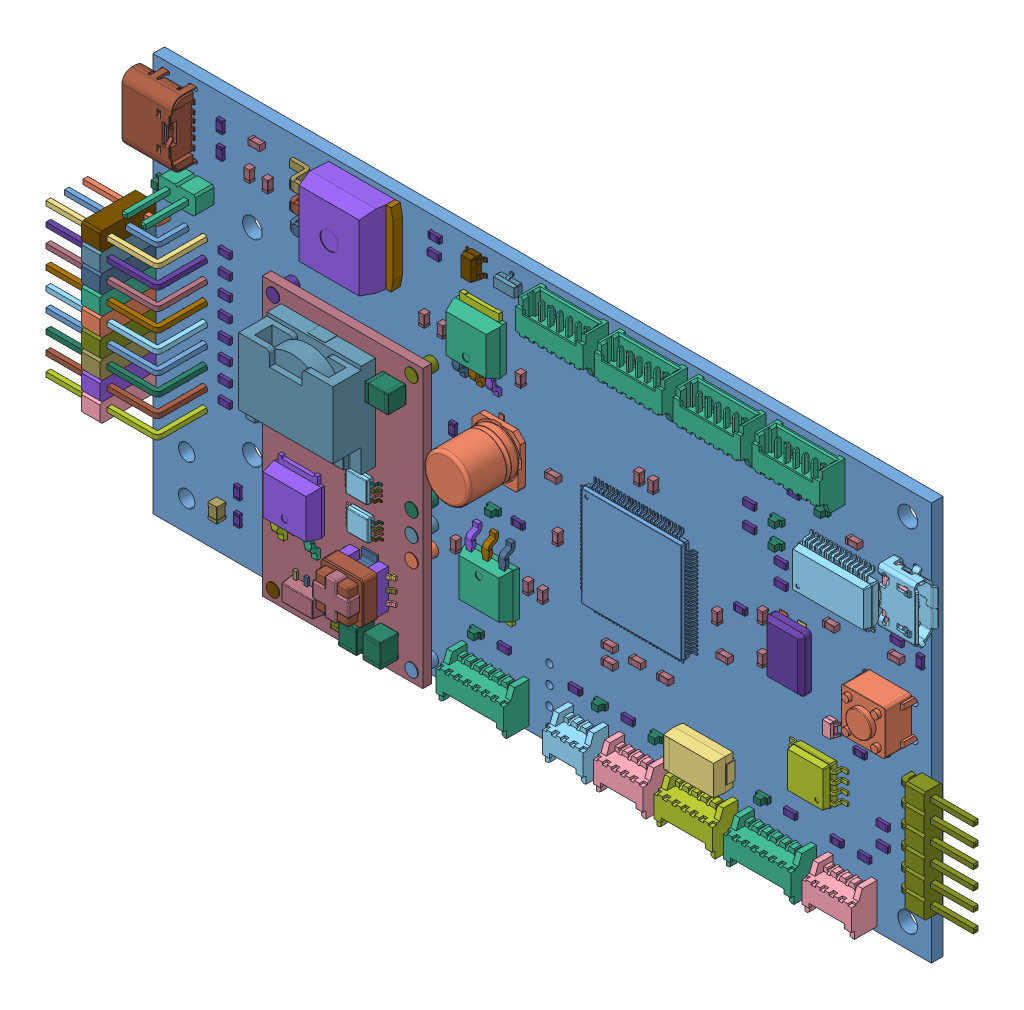
SolidWorks assembly OSAVC_simplified, configuration Default. Lengths in mm.
Overall size (122.32 54.61 12.15).
253 component instances, 116 part files, 0 mates.
Components (placement in the parent):
- OSAVC_simplified.step-1: OSAVC_simplified.step [Default] at origin size (122.32 54.61 12.15)
  - Local_CS_6c55.step-1: Local_CS_6c55.step [Default] at origin
  - Board_Geoms_6c55.step-1: Board_Geoms_6c55.step [Default] at origin size (106.68 54.61 1.6)
    - Pcb_6c55.step-1: Pcb_6c55.step [Default] at (-86.36 81.28 0) size (106.68 54.61 1.6)
    - PCB_Sketch_6c55.step-1: PCB_Sketch_6c55.step [Default] at origin
  - Step_Models_6c55.step-1: Step_Models_6c55.step [Default] at origin size (122.32 53.45 12.15)
    - Top_6c55.step-1: Top_6c55.step [Default] at origin size (122.32 53.45 12.15)
      - C2_C_Elec_63x079_00006184c965.step-1: C2_C_Elec_63x079_00006184c965.step [Default] at (47.89 -22.72 0) x (0 -1 0) z (0 0 1) size (8.61 8.6 7.7)
        - C_Elec_63x77.step-1: C_Elec_63x77.step [Default] at origin size (8.61 8.6 7.7)
        - C_Elec_63x078.step-1: C_Elec_63x078.step [Default] at origin size (0.02 0.02 0.01)
      - J4_PinHeader_3x09_P2.54mm_Horizontal036_00006184cc7d.step-1: J4_PinHeader_3x09_P2.54mm_Horizontal036_00006184cc7d.step [Default] at (6.985 -38.735 0) x (-1 0 0) z (0 0 1) size (15.44 22.86 10.62)
        - PinHeader_3x09_P2.54mm_Horizontal.step-1: PinHeader_3x09_P2.54mm_Horizontal.step [Default] at origin size (2.54 2.54 7.62)
        - PinHeader_3x09_P2.54mm_Horizontal001.step-1: PinHeader_3x09_P2.54mm_Horizontal001.step [Default] at origin size (12.9 0.64 7.13)
        - PinHeader_3x09_P2.54mm_Horizontal002.step-1: PinHeader_3x09_P2.54mm_Horizontal002.step [Default] at origin size (10.36 0.64 4.59)
        - PinHeader_3x09_P2.54mm_Horizontal003.step-1: PinHeader_3x09_P2.54mm_Horizontal003.step [Default] at origin size (15.44 0.64 9.67)
        - PinHeader_3x09_P2.54mm_Horizontal004.step-1: PinHeader_3x09_P2.54mm_Horizontal004.step [Default] at origin size (2.54 2.54 7.62)
        - PinHeader_3x09_P2.54mm_Horizontal005.step-1: PinHeader_3x09_P2.54mm_Horizontal005.step [Default] at origin size (12.9 0.64 7.13)
        - PinHeader_3x09_P2.54mm_Horizontal006.step-1: PinHeader_3x09_P2.54mm_Horizontal006.step [Default] at origin size (10.36 0.64 4.59)
        - PinHeader_3x09_P2.54mm_Horizontal007.step-1: PinHeader_3x09_P2.54mm_Horizontal007.step [Default] at origin size (15.44 0.64 9.67)
        - PinHeader_3x09_P2.54mm_Horizontal008.step-1: PinHeader_3x09_P2.54mm_Horizontal008.step [Default] at origin size (2.54 2.54 7.62)
        - PinHeader_3x09_P2.54mm_Horizontal009.step-1: PinHeader_3x09_P2.54mm_Horizontal009.step [Default] at origin size (12.9 0.64 7.13)
        - PinHeader_3x09_P2.54mm_Horizontal010.step-1: PinHeader_3x09_P2.54mm_Horizontal010.step [Default] at origin size (10.36 0.64 4.59)
        - PinHeader_3x09_P2.54mm_Horizontal011.step-1: PinHeader_3x09_P2.54mm_Horizontal011.step [Default] at origin size (15.44 0.64 9.67)
        - PinHeader_3x09_P2.54mm_Horizontal012.step-1: PinHeader_3x09_P2.54mm_Horizontal012.step [Default] at origin size (2.54 2.54 7.62)
        - PinHeader_3x09_P2.54mm_Horizontal013.step-1: PinHeader_3x09_P2.54mm_Horizontal013.step [Default] at origin size (12.9 0.64 7.13)
        - PinHeader_3x09_P2.54mm_Horizontal014.step-1: PinHeader_3x09_P2.54mm_Horizontal014.step [Default] at origin size (10.36 0.64 4.59)
        - PinHeader_3x09_P2.54mm_Horizontal015.step-1: PinHeader_3x09_P2.54mm_Horizontal015.step [Default] at origin size (15.44 0.64 9.67)
        - PinHeader_3x09_P2.54mm_Horizontal016.step-1: PinHeader_3x09_P2.54mm_Horizontal016.step [Default] at origin size (2.54 2.54 7.62)
        - PinHeader_3x09_P2.54mm_Horizontal017.step-1: PinHeader_3x09_P2.54mm_Horizontal017.step [Default] at origin size (12.9 0.64 7.13)
        - PinHeader_3x09_P2.54mm_Horizontal018.step-1: PinHeader_3x09_P2.54mm_Horizontal018.step [Default] at origin size (10.36 0.64 4.59)
        - PinHeader_3x09_P2.54mm_Horizontal019.step-1: PinHeader_3x09_P2.54mm_Horizontal019.step [Default] at origin size (15.44 0.64 9.67)
        - PinHeader_3x09_P2.54mm_Horizontal020.step-1: PinHeader_3x09_P2.54mm_Horizontal020.step [Default] at origin size (2.54 2.54 7.62)
        - PinHeader_3x09_P2.54mm_Horizontal021.step-1: PinHeader_3x09_P2.54mm_Horizontal021.step [Default] at origin size (12.9 0.64 7.13)
        - PinHeader_3x09_P2.54mm_Horizontal022.step-1: PinHeader_3x09_P2.54mm_Horizontal022.step [Default] at origin size (10.36 0.64 4.59)
        - PinHeader_3x09_P2.54mm_Horizontal023.step-1: PinHeader_3x09_P2.54mm_Horizontal023.step [Default] at origin size (15.44 0.64 9.67)
        - PinHeader_3x09_P2.54mm_Horizontal024.step-1: PinHeader_3x09_P2.54mm_Horizontal024.step [Default] at origin size (2.54 2.54 7.62)
        - PinHeader_3x09_P2.54mm_Horizontal025.step-1: PinHeader_3x09_P2.54mm_Horizontal025.step [Default] at origin size (12.9 0.64 7.13)
        - PinHeader_3x09_P2.54mm_Horizontal026.step-1: PinHeader_3x09_P2.54mm_Horizontal026.step [Default] at origin size (10.36 0.64 4.59)
        - PinHeader_3x09_P2.54mm_Horizontal027.step-1: PinHeader_3x09_P2.54mm_Horizontal027.step [Default] at origin size (15.44 0.64 9.67)
        - PinHeader_3x09_P2.54mm_Horizontal028.step-1: PinHeader_3x09_P2.54mm_Horizontal028.step [Default] at origin size (2.54 2.54 7.62)
        - PinHeader_3x09_P2.54mm_Horizontal029.step-1: PinHeader_3x09_P2.54mm_Horizontal029.step [Default] at origin size (12.9 0.64 7.13)
        - PinHeader_3x09_P2.54mm_Horizontal030.step-1: PinHeader_3x09_P2.54mm_Horizontal030.step [Default] at origin size (10.36 0.64 4.59)
        - PinHeader_3x09_P2.54mm_Horizontal031.step-1: PinHeader_3x09_P2.54mm_Horizontal031.step [Default] at origin size (15.44 0.64 9.67)
        - PinHeader_3x09_P2.54mm_Horizontal032.step-1: PinHeader_3x09_P2.54mm_Horizontal032.step [Default] at origin size (2.54 2.54 7.62)
        - PinHeader_3x09_P2.54mm_Horizontal033.step-1: PinHeader_3x09_P2.54mm_Horizontal033.step [Default] at origin size (12.9 0.64 7.13)
        - PinHeader_3x09_P2.54mm_Horizontal034.step-1: PinHeader_3x09_P2.54mm_Horizontal034.step [Default] at origin size (10.36 0.64 4.59)
        - PinHeader_3x09_P2.54mm_Horizontal035.step-1: PinHeader_3x09_P2.54mm_Horizontal035.step [Default] at origin size (15.44 0.64 9.67)
      - J13_Picoblade_horizontal_4p_00006184cca8.step-1: J13_Picoblade_horizontal_4p_00006184cca8.step [Default] at (65.405 -49.53 0) x (1 0 0) z (0 -1 0) size (6.75 5.8 5.5)
        - 530480410.step-1: 530480410.step [Default] at (1.875 1.9 3.475) x (-1 0 0) z (0 1 0) size (6.75 5.5 5.8)
      - J14_Picoblade_horizontal_3p_00006184ccd2.step-1: J14_Picoblade_horizontal_3p_00006184ccd2.step [Default] at (58.42 -49.53 0) x (1 0 0) z (0 -1 0) size (5.5 5.8 5.5)
        - 530480310.step-1: 530480310.step [Default] at (1.25 1.9 3.475) x (-1 0 0) z (0 1 0) size (5.5 5.5 5.8)
      - J15_Picoblade_horizontal_6p_00006184ccff.step-1: J15_Picoblade_horizontal_6p_00006184ccff.step [Default] at (83.185 -49.53 0) x (1 0 0) z (0 -1 0) size (9.25 5.8 5.5)
        - 530480610.step-1: 530480610.step [Default] at (3.125 1.9 3.475) x (-1 0 0) z (0 1 0) size (9.25 5.5 5.8)
      - J15_Picoblade_horizontal_6p_00006184ccff.step-2: J15_Picoblade_horizontal_6p_00006184ccff.step [Default] at (93.345 -5.08 0) x (-1 0 0) z (0 1 0) size (9.25 5.8 5.5)
        - 530480610.step-1: 530480610.step [Default] at (3.125 1.9 3.475) x (-1 0 0) z (0 1 0) size (9.25 5.5 5.8)
      - J15_Picoblade_horizontal_6p_00006184ccff.step-3: J15_Picoblade_horizontal_6p_00006184ccff.step [Default] at (82.55 -5.08 0) x (-1 0 0) z (0 1 0) size (9.25 5.8 5.5)
        - 530480610.step-1: 530480610.step [Default] at (3.125 1.9 3.475) x (-1 0 0) z (0 1 0) size (9.25 5.5 5.8)
      - J15_Picoblade_horizontal_6p_00006184ccff.step-4: J15_Picoblade_horizontal_6p_00006184ccff.step [Default] at (71.755 -5.08 0) x (-1 0 0) z (0 1 0) size (9.25 5.8 5.5)
        - 530480610.step-1: 530480610.step [Default] at (3.125 1.9 3.475) x (-1 0 0) z (0 1 0) size (9.25 5.5 5.8)
      - J20_Picoblade_horizontal_5p_00006184cddf.step-1: J20_Picoblade_horizontal_5p_00006184cddf.step [Default] at (73.66 -49.53 0) x (1 0 0) z (0 -1 0) size (8 5.8 5.5)
        - 530480510.step-1: 530480510.step [Default] at (2.5 1.9 3.475) x (-1 0 0) z (0 1 0) size (8 5.5 5.8)
      - J13_Picoblade_horizontal_4p_00006184cca8.step-2: J13_Picoblade_horizontal_4p_00006184cca8.step [Default] at (93.98 -49.53 0) x (1 0 0) z (0 -1 0) size (6.75 5.8 5.5)
        - 530480410.step-1: 530480410.step [Default] at (1.875 1.9 3.475) x (-1 0 0) z (0 1 0) size (6.75 5.5 5.8)
      - U5_CQ assembly_00006184d1ab.step-1: U5_CQ assembly_00006184d1ab.step [Default] at (28.575 -5.715 0) size (15 10 4.42)
        - a52d3816-9c39-11ed-93f0-dde97e994e83.step-1: a52d3816-9c39-11ed-93f0-dde97e994e83.step [Default] at origin size (15 10 4.42)
          - a52d3817-9c39-11ed-93f0-dde97e994e83.step-1: a52d3817-9c39-11ed-93f0-dde97e994e83.step [Default] at origin size (9.25 10 4.4)
            - a52d3817-9c39-11ed-93f0-dde97e994e83_part.step-1: a52d3817-9c39-11ed-93f0-dde97e994e83_part.step [Default] at origin size (9.25 10 4.4)
          - a52d3818-9c39-11ed-93f0-dde97e994e83.step-1: a52d3818-9c39-11ed-93f0-dde97e994e83.step [Default] at origin size (7.55 10 1.27)
            - a52d3818-9c39-11ed-93f0-dde97e994e83_part.step-1: a52d3818-9c39-11ed-93f0-dde97e994e83_part.step [Default] at origin size (7.55 10 1.27)
          - a52d3819-9c39-11ed-93f0-dde97e994e83.step-1: a52d3819-9c39-11ed-93f0-dde97e994e83.step [Default] at origin size (4.95 6.32 2.95)
            - a52d3819-9c39-11ed-93f0-dde97e994e83_part003.step-1: a52d3819-9c39-11ed-93f0-dde97e994e83_part003.step [Default] at origin size (4.95 6.32 2.95)
              - a52d3819-9c39-11ed-93f0-dde97e994e83_part.step-1: a52d3819-9c39-11ed-93f0-dde97e994e83_part.step [Default] at origin size (4.95 1.24 2.95)
              - a52d3819-9c39-11ed-93f0-dde97e994e83_part001.step-1: a52d3819-9c39-11ed-93f0-dde97e994e83_part001.step [Default] at origin size (4.95 1.24 2.95)
              - a52d3819-9c39-11ed-93f0-dde97e994e83_part002.step-1: a52d3819-9c39-11ed-93f0-dde97e994e83_part002.step [Default] at origin size (4.95 1.24 2.95)
      - J15_Picoblade_horizontal_6p_00006184ccff.step-5: J15_Picoblade_horizontal_6p_00006184ccff.step [Default] at (43.815 -49.53 0) x (1 0 0) z (0 -1 0) size (9.25 5.8 5.5)
        - 530480610.step-1: 530480610.step [Default] at (3.125 1.9 3.475) x (-1 0 0) z (0 1 0) size (9.25 5.5 5.8)
      - U1_PTN78020_00006189aa32.step-1: U1_PTN78020_00006189aa32.step [Default] at (19.304 -52.578 0) x (1 0 0) z (0 -1 0) size (22 12.09 38)
        - Board^PTN78028.step-1: Board^PTN78028.step [Default] at origin size (22 6.34 38)
          - Board^PTN78020.step-1: Board^PTN78020.step [Default] at origin size (22 1.2 38)
          - Board^PTN78021.step-1: Board^PTN78021.step [Default] at origin size (1.75 6.34 1.75)
          - Board^PTN78022.step-1: Board^PTN78022.step [Default] at origin size (1.75 6.34 1.75)
          - Board^PTN78023.step-1: Board^PTN78023.step [Default] at origin size (1.75 6.34 1.75)
          - Board^PTN78024.step-1: Board^PTN78024.step [Default] at origin size (1.75 6.34 1.75)
          - Board^PTN78025.step-1: Board^PTN78025.step [Default] at origin size (1.75 6.34 1.75)
          - Board^PTN78026.step-1: Board^PTN78026.step [Default] at origin size (1.75 6.34 1.75)
          - Board^PTN78027.step-1: Board^PTN78027.step [Default] at origin size (1.75 6.34 1.75)
        - SMTCurrentSenseTransformer011.step-1: SMTCurrentSenseTransformer011.step [Default] at origin size (7.12 5.58 6.13)
          - SMTCurrentSenseTransformer.step-1: SMTCurrentSenseTransformer.step [Default] at (13.366 2.8 -8.2501) size (0.93 0.55 0.52)
          - SMTCurrentSenseTransformer001.step-1: SMTCurrentSenseTransformer001.step [Default] at (13.366 2.8 -8.2501) size (0.93 0.55 0.52)
          - SMTCurrentSenseTransformer002.step-1: SMTCurrentSenseTransformer002.step [Default] at (13.366 2.8 -8.2501) size (0.93 0.55 0.52)
          - SMTCurrentSenseTransformer003.step-1: SMTCurrentSenseTransformer003.step [Default] at (13.366 2.8 -8.2501) size (0.93 0.55 0.52)
          - SMTCurrentSenseTransformer004.step-1: SMTCurrentSenseTransformer004.step [Default] at (13.366 2.8 -8.2501) size (0.93 0.55 0.52)
          - SMTCurrentSenseTransformer005.step-1: SMTCurrentSenseTransformer005.step [Default] at (13.366 2.8 -8.2501) size (5.27 1.76 5.27)
          - SMTCurrentSenseTransformer006.step-1: SMTCurrentSenseTransformer006.step [Default] at (13.366 2.8 -8.2501) size (2.16 1.97 1.51)
          - SMTCurrentSenseTransformer007.step-1: SMTCurrentSenseTransformer007.step [Default] at (13.366 2.8 -8.2501) size (2.16 1.97 1.51)
          - SMTCurrentSenseTransformer008.step-1: SMTCurrentSenseTransformer008.step [Default] at (13.366 2.8 -8.2501) size (5.7 3.39 5.7)
          - SMTCurrentSenseTransformer009.step-1: SMTCurrentSenseTransformer009.step [Default] at (13.366 2.8 -8.2501) size (0.93 0.55 0.52)
          - SMTCurrentSenseTransformer010.step-1: SMTCurrentSenseTransformer010.step [Default] at (13.366 2.8 -8.2501) size (5.02 1.55 5.02)
        - MSOP-018.step-1: MSOP-018.step [Default] at origin size (4.9 1.1 3)
          - MSOP-8.step-1: MSOP-8.step [Default] at (12.6175 3.1325 -15.6358) x (0 -1 0) z (-1 0 0) size (0.67 0.44 1.43)
          - MSOP-009.step-1: MSOP-009.step [Default] at (12.6175 3.1325 -15.6358) x (0 -1 0) z (-1 0 0) size (0.67 0.44 1.43)
          - MSOP-010.step-1: MSOP-010.step [Default] at (12.6175 3.1325 -15.6358) x (0 -1 0) z (-1 0 0) size (0.67 0.44 1.43)
          - MSOP-011.step-1: MSOP-011.step [Default] at (12.6175 3.1325 -15.6358) x (0 -1 0) z (-1 0 0) size (0.67 0.44 1.43)
          - MSOP-012.step-1: MSOP-012.step [Default] at (12.6175 3.1325 -15.6358) x (0 -1 0) z (-1 0 0) size (0.67 0.44 1.43)
          - MSOP-013.step-1: MSOP-013.step [Default] at (12.6175 3.1325 -15.6358) x (0 -1 0) z (-1 0 0) size (0.15 2.39 1.73)
          - MSOP-014.step-1: MSOP-014.step [Default] at (12.6175 3.1325 -15.6358) x (0 -1 0) z (-1 0 0) size (0.67 0.44 1.43)
          - MSOP-015.step-1: MSOP-015.step [Default] at (12.6175 3.1325 -15.6358) x (0 -1 0) z (-1 0 0) size (0.67 0.44 1.43)
          - MSOP-016.step-1: MSOP-016.step [Default] at (12.6175 3.1325 -15.6358) x (0 -1 0) z (-1 0 0) size (0.67 0.44 1.43)
          - MSOP-017.step-1: MSOP-017.step [Default] at (12.6175 3.1325 -15.6358) x (0 -1 0) z (-1 0 0) size (0.94 3 3.01)
        - MSOP-029.step-1: MSOP-029.step [Default] at origin size (4.9 1.1 3)
          - MSOP-8.step-1: MSOP-8.step [Default] at (12.5011 3.1325 -20.1358) x (0 -1 0) z (-1 0 0) size (0.67 0.44 1.43)
          - MSOP-009.step-1: MSOP-009.step [Default] at (12.5011 3.1325 -20.1358) x (0 -1 0) z (-1 0 0) size (0.67 0.44 1.43)
          - MSOP-010.step-1: MSOP-010.step [Default] at (12.5011 3.1325 -20.1358) x (0 -1 0) z (-1 0 0) size (0.67 0.44 1.43)
          - MSOP-011.step-1: MSOP-011.step [Default] at (12.5011 3.1325 -20.1358) x (0 -1 0) z (-1 0 0) size (0.67 0.44 1.43)
          - MSOP-012.step-1: MSOP-012.step [Default] at (12.5011 3.1325 -20.1358) x (0 -1 0) z (-1 0 0) size (0.67 0.44 1.43)
          - MSOP-013.step-1: MSOP-013.step [Default] at (12.5011 3.1325 -20.1358) x (0 -1 0) z (-1 0 0) size (0.15 2.39 1.73)
          - MSOP-014.step-1: MSOP-014.step [Default] at (12.5011 3.1325 -20.1358) x (0 -1 0) z (-1 0 0) size (0.67 0.44 1.43)
          - MSOP-015.step-1: MSOP-015.step [Default] at (12.5011 3.1325 -20.1358) x (0 -1 0) z (-1 0 0) size (0.67 0.44 1.43)
          - MSOP-016.step-1: MSOP-016.step [Default] at (12.5011 3.1325 -20.1358) x (0 -1 0) z (-1 0 0) size (0.67 0.44 1.43)
          - MSOP-017.step-1: MSOP-017.step [Default] at (12.5011 3.1325 -20.1358) x (0 -1 0) z (-1 0 0) size (0.94 3 3.01)
        - DPAK004.step-1: DPAK004.step [Default] at origin size (6.5 2.3 9.95)
          - DPAK.step-1: DPAK.step [Default] at (3.8382 3.3 -12.8868) size (1 1.4 3.06)
          - DPAK001.step-1: DPAK001.step [Default] at (3.8382 3.3 -12.8868) size (1 1.4 3.06)
          - DPAK002.step-1: DPAK002.step [Default] at (3.8382 3.3 -12.8868) size (6.5 2.3 7.05)
          - DPAK003.step-1: DPAK003.step [Default] at (3.8382 3.3 -12.8868) size (0.9 0.5 0.8)
        - SOT093.step-1: SOT093.step [Default] at origin size (4.5 1.5 4.13)
          - SOT89.step-1: SOT89.step [Default] at (4.7525 3.13 -2) x (-1 0 0) z (0 0 1) size (1.6 0.33 4.13)
          - SOT090.step-1: SOT090.step [Default] at (4.7525 3.13 -2) x (-1 0 0) z (0 0 1) size (0.47 0.33 1.48)
          - SOT091.step-1: SOT091.step [Default] at (4.7525 3.13 -2) x (-1 0 0) z (0 0 1) size (0.47 0.33 1.48)
          - SOT092.step-1: SOT092.step [Default] at (4.7525 3.13 -2) x (-1 0 0) z (0 0 1) size (4.5 1.5 2.5)
        - Coilcraft-SER1360.step-1: Coilcraft-SER1360.step [Default] at (7.55 2.8 -28.05) x (0 0 1) z (-1 0 0) size (13 5.9 12.9)
        - SMD_Capacitor_1210_1210.step-1: SMD_Capacitor_1210_1210.step [Default] at (15.94 4.04 -1.9) x (0 0 1) z (-1 0 0) size (3.2 2.5 2.5)
        - SMD_Capacitor_1210_1210.step-2: SMD_Capacitor_1210_1210.step [Default] at (12.64 4.04 -1.9) x (0 0 1) z (-1 0 0) size (3.2 2.5 2.5)
        - SMD_Capacitor_1210_1210.step-3: SMD_Capacitor_1210_1210.step [Default] at (16.6 4.04 -32.26) size (3.2 2.5 2.5)
        - SMD_Capacitor_0805_0805.step-1: SMD_Capacitor_0805_0805.step [Default] at (9.715 3.44 -1.625) x (0 0 -1) z (-1 0 0) size (2 1.3 1.25)
      - J15_Picoblade_horizontal_6p_00006184ccff.step-6: J15_Picoblade_horizontal_6p_00006184ccff.step [Default] at (60.96 -5.08 0) x (-1 0 0) z (0 1 0) size (9.25 5.8 5.5)
        - 530480610.step-1: 530480610.step [Default] at (3.125 1.9 3.475) x (-1 0 0) z (0 1 0) size (9.25 5.5 5.8)
      - Y1_SMD_crystal005_0000618b2749.step-1: Y1_SMD_crystal005_0000618b2749.step [Default] at (87.757 -27.051 0) x (0 1 0) z (0 0 1) size (8.22 5.2 1.5)
        - SMD_crystal.step-1: SMD_crystal.step [Default] at origin size (7.5 5.2 1.4)
        - SMD_crystal001.step-1: SMD_crystal001.step [Default] at origin size (1.92 1.12 0.1)
        - SMD_crystal002.step-1: SMD_crystal002.step [Default] at origin size (1.92 1.12 0.1)
        - SMD_crystal003.step-1: SMD_crystal003.step [Default] at origin size (1.92 1.12 0.1)
        - SMD_crystal004.step-1: SMD_crystal004.step [Default] at origin size (1.92 1.12 0.1)
      - J3_10118193003_0000618b348a.step-1: J3_10118193003_0000618b348a.step [Default] at (104.805 -12.065 0) x (0 1 0) z (1 0 0) size (7.87 3.61 5.71)
        - 10118193002.step-1: 10118193002.step [Default] at origin size (7.87 3.61 5.71)
          - 10118193.step-1: 10118193.step [Default] at (-0.19 0.055 -0.3676) size (6.89 2.35 4.32)
          - 10118193001.step-1: 10118193001.step [Default] at (-0.19 0.055 -0.3676) size (7.87 3.61 5.67)
      - U3_CQ assembly_0000618ecb8d.step-1: U3_CQ assembly_0000618ecb8d.step [Default] at (46.99 -38.8526 0) x (0 -1 0) z (0 0 1) size (9.9 6.5 2.32)
        - 98f8d7e0-9c39-11ed-93f0-dde97e994e83.step-1: 98f8d7e0-9c39-11ed-93f0-dde97e994e83.step [Default] at origin size (9.9 6.5 2.32)
          - 98f8d7e1-9c39-11ed-93f0-dde97e994e83.step-1: 98f8d7e1-9c39-11ed-93f0-dde97e994e83.step [Default] at origin size (6.22 6.5 2.3)
            - 98f8d7e1-9c39-11ed-93f0-dde97e994e83_part.step-1: 98f8d7e1-9c39-11ed-93f0-dde97e994e83_part.step [Default] at origin size (6.22 6.5 2.3)
          - 98f8d7e2-9c39-11ed-93f0-dde97e994e83.step-1: 98f8d7e2-9c39-11ed-93f0-dde97e994e83.step [Default] at origin size (5.24 5.4 0.5)
            - 98f8d7e2-9c39-11ed-93f0-dde97e994e83_part.step-1: 98f8d7e2-9c39-11ed-93f0-dde97e994e83_part.step [Default] at origin size (5.24 5.4 0.5)
          - 98f8d7e3-9c39-11ed-93f0-dde97e994e83.step-1: 98f8d7e3-9c39-11ed-93f0-dde97e994e83.step [Default] at origin size (3.55 5.55 1.44)
            - 98f8d7e3-9c39-11ed-93f0-dde97e994e83_part003.step-1: 98f8d7e3-9c39-11ed-93f0-dde97e994e83_part003.step [Default] at origin size (3.55 5.55 1.44)
              - 98f8d7e3-9c39-11ed-93f0-dde97e994e83_part.step-1: 98f8d7e3-9c39-11ed-93f0-dde97e994e83_part.step [Default] at origin size (3.55 0.99 1.44)
              - 98f8d7e3-9c39-11ed-93f0-dde97e994e83_part001.step-1: 98f8d7e3-9c39-11ed-93f0-dde97e994e83_part001.step [Default] at origin size (3.55 0.99 1.44)
              - 98f8d7e3-9c39-11ed-93f0-dde97e994e83_part002.step-1: 98f8d7e3-9c39-11ed-93f0-dde97e994e83_part002.step [Default] at origin size (3.55 0.99 1.44)
      - U3_CQ assembly_0000618ecb8d.step-2: U3_CQ assembly_0000618ecb8d.step [Default] at (45.212 -10.8044 0) x (0 1 0) z (0 0 1) size (9.9 6.5 2.32)
        - 98f8d7e0-9c39-11ed-93f0-dde97e994e83.step-1: 98f8d7e0-9c39-11ed-93f0-dde97e994e83.step [Default] at origin size (9.9 6.5 2.32)
          - 98f8d7e1-9c39-11ed-93f0-dde97e994e83.step-1: 98f8d7e1-9c39-11ed-93f0-dde97e994e83.step [Default] at origin size (6.22 6.5 2.3)
            - 98f8d7e1-9c39-11ed-93f0-dde97e994e83_part.step-1: 98f8d7e1-9c39-11ed-93f0-dde97e994e83_part.step [Default] at origin size (6.22 6.5 2.3)
          - 98f8d7e2-9c39-11ed-93f0-dde97e994e83.step-1: 98f8d7e2-9c39-11ed-93f0-dde97e994e83.step [Default] at origin size (5.24 5.4 0.5)
            - 98f8d7e2-9c39-11ed-93f0-dde97e994e83_part.step-1: 98f8d7e2-9c39-11ed-93f0-dde97e994e83_part.step [Default] at origin size (5.24 5.4 0.5)
          - 98f8d7e3-9c39-11ed-93f0-dde97e994e83.step-1: 98f8d7e3-9c39-11ed-93f0-dde97e994e83.step [Default] at origin size (3.55 5.55 1.44)
            - 98f8d7e3-9c39-11ed-93f0-dde97e994e83_part003.step-1: 98f8d7e3-9c39-11ed-93f0-dde97e994e83_part003.step [Default] at origin size (3.55 5.55 1.44)
              - 98f8d7e3-9c39-11ed-93f0-dde97e994e83_part.step-1: 98f8d7e3-9c39-11ed-93f0-dde97e994e83_part.step [Default] at origin size (3.55 0.99 1.44)
              - 98f8d7e3-9c39-11ed-93f0-dde97e994e83_part001.step-1: 98f8d7e3-9c39-11ed-93f0-dde97e994e83_part001.step [Default] at origin size (3.55 0.99 1.44)
              - 98f8d7e3-9c39-11ed-93f0-dde97e994e83_part002.step-1: 98f8d7e3-9c39-11ed-93f0-dde97e994e83_part002.step [Default] at origin size (3.55 0.99 1.44)
      - J23_USB4125-GF-A_000061969e33.step-1: J23_USB4125-GF-A_000061969e33.step [Default] at (-0.96 -5.58 0) x (0 -1 0) z (-1 0 0) size (8.95 4.43 7.12)
        - USB4125-GF-A_PART1.step-1: USB4125-GF-A_PART1.step [Default] at origin size (8.95 4.43 7.12)
      - C1_C_0805_2012Metric_00006184c954.step-1: C1_C_0805_2012Metric_00006184c954.step [Default] at (9.39 -49.22 0) x (0 -1 0) z (0 0 1) size (2 1.25 1.25)
      - C3_C_0603_1608Metric_00006184c976.step-1: C3_C_0603_1608Metric_00006184c976.step [Default] at (50.8 -12.954 0) x (0 1 0) z (0 0 1) size (1.6 0.8 0.8)
      - C3_C_0603_1608Metric_00006184c976.step-2: C3_C_0603_1608Metric_00006184c976.step [Default] at (40.14 -12.47 0) x (0 1 0) z (0 0 1) size (1.6 0.8 0.8)
      - C3_C_0603_1608Metric_00006184c976.step-3: C3_C_0603_1608Metric_00006184c976.step [Default] at (41.91 -37.084 0) x (0 -1 0) z (0 0 1) size (1.6 0.8 0.8)
      - C3_C_0603_1608Metric_00006184c976.step-4: C3_C_0603_1608Metric_00006184c976.step [Default] at (51.816 -37.084 0) x (0 -1 0) z (0 0 1) size (1.6 0.8 0.8)
      - C3_C_0603_1608Metric_00006184c976.step-5: C3_C_0603_1608Metric_00006184c976.step [Default] at (14.605 -3.175 0) x (-1 0 0) z (0 0 1) size (1.6 0.8 0.8)
      - C3_C_0603_1608Metric_00006184c976.step-6: C3_C_0603_1608Metric_00006184c976.step [Default] at (16.14 -7.22 0) x (0 1 0) z (0 0 1) size (1.6 0.8 0.8)
      - C3_C_0603_1608Metric_00006184c976.step-7: C3_C_0603_1608Metric_00006184c976.step [Default] at (55.88 -29.21 0) x (0 1 0) z (0 0 1) size (1.6 0.8 0.8)
      - C3_C_0603_1608Metric_00006184c976.step-8: C3_C_0603_1608Metric_00006184c976.step [Default] at (70.612 -38.608 0) x (-1 0 0) z (0 0 1) size (1.6 0.8 0.8)
      - C3_C_0603_1608Metric_00006184c976.step-9: C3_C_0603_1608Metric_00006184c976.step [Default] at (67.056 -16.51 0) x (0 1 0) z (0 0 1) size (1.6 0.8 0.8)
      - C3_C_0603_1608Metric_00006184c976.step-10: C3_C_0603_1608Metric_00006184c976.step [Default] at (62.992 -38.608 0) size (1.6 0.8 0.8)
      - C3_C_0603_1608Metric_00006184c976.step-11: C3_C_0603_1608Metric_00006184c976.step [Default] at (62.992 -40.64 0) size (1.6 0.8 0.8)
      - C3_C_0603_1608Metric_00006184c976.step-12: C3_C_0603_1608Metric_00006184c976.step [Default] at (13.64 -7.22 0) x (0 1 0) z (0 0 1) size (1.6 0.8 0.8)
      - C3_C_0603_1608Metric_00006184c976.step-13: C3_C_0603_1608Metric_00006184c976.step [Default] at (37.592 -12.446 0) x (0 1 0) z (0 0 1) size (1.6 0.8 0.8)
      - C3_C_0603_1608Metric_00006184c976.step-14: C3_C_0603_1608Metric_00006184c976.step [Default] at (53.848 -37.084 0) x (0 -1 0) z (0 0 1) size (1.6 0.8 0.8)
      - D6_SOT_23_00006184cb73.step-1: D6_SOT_23_00006184cb73.step [Default] at (14.605 -34.29 0) size (2.5 3 1.2)
      - D6_SOT_23_00006184cb73.step-2: D6_SOT_23_00006184cb73.step [Default] at (14.605 -29.845 0) size (2.5 3 1.2)
      - D8_LED_0603_1608Metric_00006184cb9b.step-1: D8_LED_0603_1608Metric_00006184cb9b.step [Default] at (1.27 -14.478 0) x (0 1 0) z (0 0 1) size (1.6 0.8 1.1)
      - D8_LED_0603_1608Metric_00006184cb9b.step-2: D8_LED_0603_1608Metric_00006184cb9b.step [Default] at (61.64 -46.22 0) x (-1 0 0) z (0 0 1) size (1.6 0.8 1.1)
      - D8_LED_0603_1608Metric_00006184cb9b.step-3: D8_LED_0603_1608Metric_00006184cb9b.step [Default] at (44.64 -46.22 0) size (1.6 0.8 1.1)
      - D8_LED_0603_1608Metric_00006184cb9b.step-4: D8_LED_0603_1608Metric_00006184cb9b.step [Default] at (83.89 -46.22 0) size (1.6 0.8 1.1)
      - D8_LED_0603_1608Metric_00006184cb9b.step-5: D8_LED_0603_1608Metric_00006184cb9b.step [Default] at (69.39 -46.22 0) x (-1 0 0) z (0 0 1) size (1.6 0.8 1.1)
      - D8_LED_0603_1608Metric_00006184cb9b.step-6: D8_LED_0603_1608Metric_00006184cb9b.step [Default] at (92.14 -7.97 0) x (-1 0 0) z (0 0 1) size (1.6 0.8 1.1)
      - J2_PinHeader_1x06_P254mm_Horizontal_00006184cc31.step-1: J2_PinHeader_1x06_P254mm_Horizontal_00006184cc31.step [Default] at (104.14 -33.655 0) size (10.36 15.24 5.54)
      - D6_SOT_23_00006184cb73.step-3: D6_SOT_23_00006184cb73.step [Default] at (49.276 -2.54 0) x (0 1 0) z (0 0 1) size (2.5 3 1.2)
      - R3_R_0603_1608Metric_00006184ceac.step-1: R3_R_0603_1608Metric_00006184ceac.step [Default] at (38.81 -4.318 0) size (1.6 0.8 0.45)
      - R3_R_0603_1608Metric_00006184ceac.step-2: R3_R_0603_1608Metric_00006184ceac.step [Default] at (100.33 -41.275 0) x (-1 0 0) z (0 0 1) size (1.6 0.8 0.45)
      - R3_R_0603_1608Metric_00006184ceac.step-3: R3_R_0603_1608Metric_00006184ceac.step [Default] at (100.33 -43.815 0) x (-1 0 0) z (0 0 1) size (1.6 0.8 0.45)
      - R3_R_0603_1608Metric_00006184ceac.step-4: R3_R_0603_1608Metric_00006184ceac.step [Default] at (97.155 -34.29 0) x (-1 0 0) z (0 0 1) size (1.6 0.8 0.45)
      - R3_R_0603_1608Metric_00006184ceac.step-5: R3_R_0603_1608Metric_00006184ceac.step [Default] at (100.33 -32.385 0) size (1.6 0.8 0.45)
      - R3_R_0603_1608Metric_00006184ceac.step-6: R3_R_0603_1608Metric_00006184ceac.step [Default] at (80.772 -25.4 0) size (1.6 0.8 0.45)
      - R3_R_0603_1608Metric_00006184ceac.step-7: R3_R_0603_1608Metric_00006184ceac.step [Default] at (86.36 -19.685 0) x (-1 0 0) z (0 0 1) size (1.6 0.8 0.45)
      - R3_R_0603_1608Metric_00006184ceac.step-8: R3_R_0603_1608Metric_00006184ceac.step [Default] at (86.36 -17.145 0) x (-1 0 0) z (0 0 1) size (1.6 0.8 0.45)
      - R3_R_0603_1608Metric_00006184ceac.step-9: R3_R_0603_1608Metric_00006184ceac.step [Default] at (3.81 -15.494 0) x (-1 0 0) z (0 0 1) size (1.6 0.8 0.45)
      - R3_R_0603_1608Metric_00006184ceac.step-10: R3_R_0603_1608Metric_00006184ceac.step [Default] at (10.16 -26.035 0) size (1.6 0.8 0.45)
      - R3_R_0603_1608Metric_00006184ceac.step-11: R3_R_0603_1608Metric_00006184ceac.step [Default] at (10.16 -23.495 0) size (1.6 0.8 0.45)
      - R3_R_0603_1608Metric_00006184ceac.step-12: R3_R_0603_1608Metric_00006184ceac.step [Default] at (10.16 -20.955 0) size (1.6 0.8 0.45)
      - R3_R_0603_1608Metric_00006184ceac.step-13: R3_R_0603_1608Metric_00006184ceac.step [Default] at (10.16 -18.415 0) size (1.6 0.8 0.45)
      - R3_R_0603_1608Metric_00006184ceac.step-14: R3_R_0603_1608Metric_00006184ceac.step [Default] at (58.14 -46.22 0) size (1.6 0.8 0.45)
      - R3_R_0603_1608Metric_00006184ceac.step-15: R3_R_0603_1608Metric_00006184ceac.step [Default] at (48.39 -46.22 0) x (-1 0 0) z (0 0 1) size (1.6 0.8 0.45)
      - R3_R_0603_1608Metric_00006184ceac.step-16: R3_R_0603_1608Metric_00006184ceac.step [Default] at (65.39 -46.22 0) size (1.6 0.8 0.45)
      - R3_R_0603_1608Metric_00006184ceac.step-17: R3_R_0603_1608Metric_00006184ceac.step [Default] at (88.14 -7.97 0) size (1.6 0.8 0.45)
      - R3_R_0603_1608Metric_00006184ceac.step-18: R3_R_0603_1608Metric_00006184ceac.step [Default] at (97.79 -46.355 0) x (-1 0 0) z (0 0 1) size (1.6 0.8 0.45)
      - R3_R_0603_1608Metric_00006184ceac.step-19: R3_R_0603_1608Metric_00006184ceac.step [Default] at (93.98 -46.355 0) x (-1 0 0) z (0 0 1) size (1.6 0.8 0.45)
      - R3_R_0603_1608Metric_00006184ceac.step-20: R3_R_0603_1608Metric_00006184ceac.step [Default] at (10.16 -36.195 0) x (-1 0 0) z (0 0 1) size (1.6 0.8 0.45)
      - R3_R_0603_1608Metric_00006184ceac.step-21: R3_R_0603_1608Metric_00006184ceac.step [Default] at (10.16 -31.115 0) x (-1 0 0) z (0 0 1) size (1.6 0.8 0.45)
      - R3_R_0603_1608Metric_00006184ceac.step-22: R3_R_0603_1608Metric_00006184ceac.step [Default] at (10.16 -28.575 0) x (-1 0 0) z (0 0 1) size (1.6 0.8 0.45)
      - U4_SOT_23_5_00006184d16f.step-1: U4_SOT_23_5_00006184d16f.step [Default] at (44.45 -2.54 0) size (2.8 2.9 1.55)
      - U6_TQFP_100_14x14mm_P05mm_00006184d23a.step-1: U6_TQFP_100_14x14mm_P05mm_00006184d23a.step [Default] at (66.675 -27.94 0) size (16 16 1.1)
      - SW1_SW_PUSH_6mm_h4.3mm_000061854ea1.step-1: SW1_SW_PUSH_6mm_h4.3mm_000061854ea1.step [Default] at (97.79 -24.765 0) size (7.17 6 7.8)
      - C3_C_0603_1608Metric_00006184c976.step-15: C3_C_0603_1608Metric_00006184c976.step [Default] at (55.245 -22.352 0) x (-1 0 0) z (0 0 1) size (1.6 0.8 0.8)
      - C3_C_0603_1608Metric_00006184c976.step-16: C3_C_0603_1608Metric_00006184c976.step [Default] at (78.74 -32.004 0) size (1.6 0.8 0.8)
      - C3_C_0603_1608Metric_00006184c976.step-17: C3_C_0603_1608Metric_00006184c976.step [Default] at (68.961 -16.51 0) x (0 1 0) z (0 0 1) size (1.6 0.8 0.8)
      - C24_CP_EIA_7343_30_AVX_N_00006185f6b5.step-1: C24_CP_EIA_7343_30_AVX_N_00006185f6b5.step [Default] at (76.2 -45.085 0) size (7.3 4.3 2.8)
      - R3_R_0603_1608Metric_00006184ceac.step-23: R3_R_0603_1608Metric_00006184ceac.step [Default] at (41.39 -23.72 0) x (0 1 0) z (0 0 1) size (1.6 0.8 0.45)
      - C3_C_0603_1608Metric_00006184c976.step-18: C3_C_0603_1608Metric_00006184c976.step [Default] at (96.52 -9.525 0) x (-1 0 0) z (0 0 1) size (1.6 0.8 0.8)
      - R3_R_0603_1608Metric_00006184ceac.step-24: R3_R_0603_1608Metric_00006184ceac.step [Default] at (82.042 -15.113 0) size (1.6 0.8 0.45)
      - R3_R_0603_1608Metric_00006184ceac.step-25: R3_R_0603_1608Metric_00006184ceac.step [Default] at (102.235 -18.415 0) x (-1 0 0) z (0 0 1) size (1.6 0.8 0.45)
      - R3_R_0603_1608Metric_00006184ceac.step-26: R3_R_0603_1608Metric_00006184ceac.step [Default] at (105.41 -19.304 0) x (0 -1 0) z (0 0 1) size (1.6 0.8 0.45)
      - R3_R_0603_1608Metric_00006184ceac.step-27: R3_R_0603_1608Metric_00006184ceac.step [Default] at (82.042 -12.319 0) size (1.6 0.8 0.45)
      - D8_LED_0603_1608Metric_00006184cb9b.step-7: D8_LED_0603_1608Metric_00006184cb9b.step [Default] at (85.852 -15.113 0) x (-1 0 0) z (0 0 1) size (1.6 0.8 1.1)
      - D8_LED_0603_1608Metric_00006184cb9b.step-8: D8_LED_0603_1608Metric_00006184cb9b.step [Default] at (85.852 -12.319 0) x (-1 0 0) z (0 0 1) size (1.6 0.8 1.1)
      - D3_SOT_323_SC_70_000061899956.step-1: D3_SOT_323_SC_70_000061899956.step [Default] at (93.345 -33.02 0) x (-1 0 0) z (0 0 1) size (2 2 1.05)
      - C3_C_0603_1608Metric_00006184c976.step-19: C3_C_0603_1608Metric_00006184c976.step [Default] at (93.345 -20.955 0) size (1.6 0.8 0.8)
      - U7_SSOP_28_53x102mm_P065mm_0000618a0f45.step-1: U7_SSOP_28_53x102mm_P065mm_0000618a0f45.step [Default] at (94.615 -15.24 0) x (0 1 0) z (0 0 1) size (7.8 10.2 2.1)
      - C3_C_0603_1608Metric_00006184c976.step-20: C3_C_0603_1608Metric_00006184c976.step [Default] at (102.235 -20.32 0) x (-1 0 0) z (0 0 1) size (1.6 0.8 0.8)
      - C3_C_0603_1608Metric_00006184c976.step-21: C3_C_0603_1608Metric_00006184c976.step [Default] at (83.947 -24.511 0) x (0 1 0) z (0 0 1) size (1.6 0.8 0.8)
      - C3_C_0603_1608Metric_00006184c976.step-22: C3_C_0603_1608Metric_00006184c976.step [Default] at (83.947 -29.591 0) x (0 -1 0) z (0 0 1) size (1.6 0.8 0.8)
      - C3_C_0603_1608Metric_00006184c976.step-23: C3_C_0603_1608Metric_00006184c976.step [Default] at (77.724 -27.686 0) x (0 1 0) z (0 0 1) size (1.6 0.8 0.8)
      - R3_R_0603_1608Metric_00006184ceac.step-28: R3_R_0603_1608Metric_00006184ceac.step [Default] at (97.155 -32.385 0) size (1.6 0.8 0.45)
      - C3_C_0603_1608Metric_00006184c976.step-24: C3_C_0603_1608Metric_00006184c976.step [Default] at (66.802 -38.608 0) x (-1 0 0) z (0 0 1) size (1.6 0.8 0.8)
      - R3_R_0603_1608Metric_00006184ceac.step-29: R3_R_0603_1608Metric_00006184ceac.step [Default] at (11.89 -45.97 0) x (0 -1 0) z (0 0 1) size (1.6 0.8 0.45)
      - R3_R_0603_1608Metric_00006184ceac.step-30: R3_R_0603_1608Metric_00006184ceac.step [Default] at (11.89 -49.22 0) x (0 -1 0) z (0 0 1) size (1.6 0.8 0.45)
      - J5_PinHeader_1x02_P254mm_Vertical_0000618bbe19.step-1: J5_PinHeader_1x02_P254mm_Vertical_0000618bbe19.step [Default] at (7.112 -12.7 0) x (0 -1 0) z (0 0 1) size (2.54 5.08 11.54)
      - R3_R_0603_1608Metric_00006184ceac.step-31: R3_R_0603_1608Metric_00006184ceac.step [Default] at (38.91 -2.198 0) x (-1 0 0) z (0 0 1) size (1.6 0.8 0.45)
      - R3_R_0603_1608Metric_00006184ceac.step-32: R3_R_0603_1608Metric_00006184ceac.step [Default] at (50.292 -30.48 0) x (-1 0 0) z (0 0 1) size (1.6 0.8 0.45)
      - D8_LED_0603_1608Metric_00006184cb9b.step-9: D8_LED_0603_1608Metric_00006184cb9b.step [Default] at (46.99 -30.48 0) size (1.6 0.8 1.1)
      - R3_R_0603_1608Metric_00006184ceac.step-33: R3_R_0603_1608Metric_00006184ceac.step [Default] at (9.525 -6.85 0) x (0 -1 0) z (0 0 1) size (1.6 0.8 0.45)
      - R3_R_0603_1608Metric_00006184ceac.step-34: R3_R_0603_1608Metric_00006184ceac.step [Default] at (9.525 -3.675 0) x (0 1 0) z (0 0 1) size (1.6 0.8 0.45)
      - R3_R_0603_1608Metric_00006184ceac.step-35: R3_R_0603_1608Metric_00006184ceac.step [Default] at (10.16 -33.655 0) x (-1 0 0) z (0 0 1) size (1.6 0.8 0.45)
      - U9_SOIJ_8_53x53mm_P127mm_000061dd964d.step-1: U9_SOIJ_8_53x53mm_P127mm_000061dd964d.step [Default] at (91.39 -39.47 0) x (-1 0 0) z (0 0 1) size (7.94 5.3 2.01)
      - R3_R_0603_1608Metric_00006184ceac.step-36: R3_R_0603_1608Metric_00006184ceac.step [Default] at (87.64 -46.22 0) x (-1 0 0) z (0 0 1) size (1.6 0.8 0.45)
